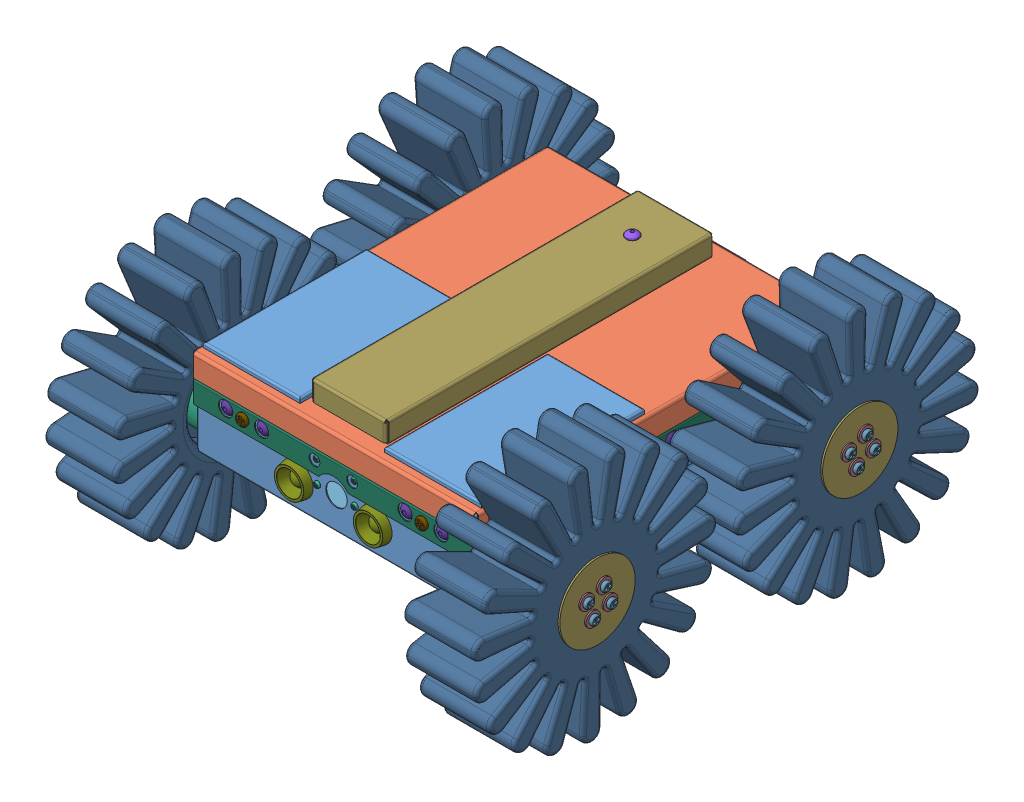
SolidWorks assembly GB0814, configuration Default. Lengths in mm. (continued)
Mates (geometry in assembly coordinates): (continued)
- Concentric111: concentric anti-aligned: cylinder of servo.fixture-1 through (144.387 0 47.956) axis (0 1 0) radius 2; cylinder of 4mm.rivet-1 through (144.387 -2.1069 47.956) axis (0 -1 0) radius 1.9261
- Concentric112: concentric anti-aligned: cylinder of servo.fixture-1 through (144.387 0 27.956) axis (0 1 0) radius 2; cylinder of 4mm.rivet-3 through (144.387 -2.1069 27.956) axis (0 -1 0) radius 1.9261
- Concentric113: concentric anti-aligned: cylinder of servo.fixture-1 through (144.387 0 7.956) axis (0 1 0) radius 2; cylinder of 4mm.rivet-2 through (144.387 -2.1069 7.956) axis (0 -1 0) radius 1.9261
- Coincident131: coincident anti-aligned: plane of case.bottom-1 through (0 -0.5 0) normal (0 -1 0); plane of 4mm.rivet-2 through (144.3664 -0.5 7.9425) normal (0 1 0)
- Coincident132: coincident anti-aligned: plane of case.bottom-1 through (0 -0.5 0) normal (0 -1 0); plane of 4mm.rivet-3 through (144.3664 -0.5 27.9425) normal (0 1 0)
- Coincident133: coincident anti-aligned: plane of case.bottom-1 through (0 -0.5 0) normal (0 -1 0); plane of 4mm.rivet-1 through (144.3664 -0.5 47.9425) normal (0 1 0)
- Coincident134: coincident anti-aligned: plane of case.bottom-1 through (0 0 0) normal (0 1 0); plane of servo.fixture-2 through (135.0187 0 151.7511) normal (0 -1 0)
- Coincident135: coincident anti-aligned: plane of SM4315R-4 through (137.0187 21 161.9111) normal (-1 0 0); plane of servo.fixture-2 through (137.0187 19 151.7511) normal (1 0 0)
- Concentric114: concentric aligned: cylinder of SM4315R-4 through (139.4 26.08 175.8811) axis (-1 0 0) radius 2.2606; cylinder of servo.fixture-2 through (153.0188 26.08 175.8811) axis (-1 0 0) radius 1.5
- Concentric115: concentric anti-aligned: cylinder of SM4315R-4 through (139.4 26.08 175.8811) axis (-1 0 0) radius 2.2606; cylinder of m3.screw.10mm-12 through (129.4 26.08 175.8811) axis (1 0 0) radius 1.5
- Coincident136: coincident anti-aligned: plane of SM4315R-4 through (139.4 21 161.9111) normal (1 0 0); plane of m3.screw.10mm-12 through (139.4 26.0936 175.8675) normal (-1 0 0)
- Concentric116: concentric anti-aligned: cylinder of SM4315R-4 through (139.4 15.92 175.8811) axis (-1 0 0) radius 2.2606; cylinder of m3.screw.10mm-9 through (129.4 15.92 175.8811) axis (1 0 0) radius 1.5
- Coincident137: coincident anti-aligned: plane of SM4315R-4 through (139.4 21 161.9111) normal (1 0 0); plane of m3.screw.10mm-9 through (139.4 15.9336 175.8675) normal (-1 0 0)
- Concentric117: concentric anti-aligned: cylinder of SM4315R-4 through (139.4 15.92 127.6211) axis (-1 0 0) radius 2.2606; cylinder of m3.screw.10mm-10 through (129.4 15.92 127.6211) axis (1 0 0) radius 1.5
- Concentric118: concentric anti-aligned: cylinder of SM4315R-4 through (139.4 26.08 127.6211) axis (-1 0 0) radius 2.2606; cylinder of m3.screw.10mm-11 through (129.4 26.08 127.6211) axis (1 0 0) radius 1.5
- Coincident138: coincident anti-aligned: plane of SM4315R-4 through (139.4 21 161.9111) normal (1 0 0); plane of m3.screw.10mm-11 through (139.4 26.0936 127.6075) normal (-1 0 0)
- Coincident139: coincident anti-aligned: plane of SM4315R-4 through (139.4 21 161.9111) normal (1 0 0); plane of m3.screw.10mm-10 through (139.4 15.9336 127.6075) normal (-1 0 0)
- Concentric119: concentric anti-aligned: cylinder of m3.screw.10mm-11 through (129.4 26.08 127.6211) axis (1 0 0) radius 1.5; cylinder of self.stop.nut.m3-25 through (135.0187 26.08 127.6211) axis (-1 0 0) radius 1.5
- Coincident140: coincident anti-aligned: plane of servo.fixture-2 through (135.0187 19 151.7511) normal (-1 0 0); plane of self.stop.nut.m3-25 through (135.0187 26.08 127.6211) normal (1 0 0)
- Concentric120: concentric anti-aligned: cylinder of m3.screw.10mm-10 through (129.4 15.92 127.6211) axis (1 0 0) radius 1.5; cylinder of self.stop.nut.m3-23 through (135.0187 15.92 127.6211) axis (-1 0 0) radius 1.5
- Coincident141: coincident anti-aligned: plane of servo.fixture-2 through (135.0187 19 151.7511) normal (-1 0 0); plane of self.stop.nut.m3-23 through (135.0187 15.92 127.6211) normal (1 0 0)
- Concentric121: concentric anti-aligned: cylinder of m3.screw.10mm-9 through (129.4 15.92 175.8811) axis (1 0 0) radius 1.5; cylinder of self.stop.nut.m3-24 through (135.0187 15.92 175.8811) axis (-1 0 0) radius 1.5
- Coincident142: coincident anti-aligned: plane of servo.fixture-2 through (135.0187 19 151.7511) normal (-1 0 0); plane of self.stop.nut.m3-24 through (135.0187 15.92 175.8811) normal (1 0 0)
- Concentric122: concentric anti-aligned: cylinder of m3.screw.10mm-12 through (129.4 26.08 175.8811) axis (1 0 0) radius 1.5; cylinder of self.stop.nut.m3-22 through (135.0187 26.08 175.8811) axis (-1 0 0) radius 1.5
- Coincident143: coincident anti-aligned: plane of servo.fixture-2 through (135.0187 19 151.7511) normal (-1 0 0); plane of self.stop.nut.m3-22 through (135.0187 26.08 175.8811) normal (1 0 0)
- Concentric123: concentric anti-aligned: cylinder of servo.fixture-2 through (144.387 0 171.7511) axis (0 1 0) radius 2; cylinder of 4mm.rivet-6 through (144.387 -2.1069 171.7511) axis (0 -1 0) radius 1.9261
- Concentric124: concentric anti-aligned: cylinder of servo.fixture-2 through (144.387 0 151.7511) axis (0 1 0) radius 2; cylinder of 4mm.rivet-5 through (144.387 -2.1069 151.7511) axis (0 -1 0) radius 1.9261
- Concentric125: concentric anti-aligned: cylinder of servo.fixture-2 through (144.387 0 131.7511) axis (0 1 0) radius 2; cylinder of 4mm.rivet-4 through (144.387 -2.1069 131.7511) axis (0 -1 0) radius 1.9261
- Coincident144: coincident anti-aligned: plane of case.bottom-1 through (0 -0.5 0) normal (0 -1 0); plane of 4mm.rivet-6 through (144.3664 -0.5 171.7376) normal (0 1 0)
- Coincident145: coincident anti-aligned: plane of case.bottom-1 through (0 -0.5 0) normal (0 -1 0); plane of 4mm.rivet-4 through (144.3664 -0.5 131.7376) normal (0 1 0)
- Coincident146: coincident anti-aligned: plane of case.bottom-1 through (0 -0.5 0) normal (0 -1 0); plane of 4mm.rivet-5 through (144.3664 -0.5 151.7376) normal (0 1 0)
- Coincident147: coincident anti-aligned: plane of case.bottom-1 through (0 0 0) normal (0 1 0); plane of servo.fixture-3 through (19.9812 0 151.7511) normal (0 -1 0)
- Coincident148: coincident anti-aligned: plane of SM4315R-1 through (17.9812 21 161.9111) normal (1 0 0); plane of servo.fixture-3 through (17.9812 19 151.7511) normal (-1 0 0)
- Concentric126: concentric aligned: cylinder of SM4315R-1 through (15.6 26.08 127.6211) axis (1 0 0) radius 2.2606; cylinder of servo.fixture-3 through (1.9812 26.08 127.6211) axis (1 0 0) radius 1.5
- Coincident149: coincident anti-aligned: plane of case.bottom-1 through (0 0 0) normal (0 1 0); plane of servo.fixture-4 through (19.9812 0 27.956) normal (0 -1 0)
- Coincident150: coincident anti-aligned: plane of SM4315R-2 through (17.9812 21 17.796) normal (1 0 0); plane of servo.fixture-4 through (17.9812 19 27.956) normal (-1 0 0)
- Concentric127: concentric aligned: cylinder of SM4315R-2 through (15.6 26.08 3.826) axis (1 0 0) radius 2.2606; cylinder of servo.fixture-4 through (1.9812 26.08 3.826) axis (1 0 0) radius 1.5
- Coincident151: coincident anti-aligned: plane of case.bottom-1 through (0 -0.5 0) normal (0 -1 0); plane of 4mm.rivet-9 through (10.5923 -0.5 47.9425) normal (0 1 0)
- Coincident152: coincident anti-aligned: plane of case.bottom-1 through (0 -0.5 0) normal (0 -1 0); plane of 4mm.rivet-8 through (10.5923 -0.5 27.9425) normal (0 1 0)
- Coincident153: coincident anti-aligned: plane of case.bottom-1 through (0 -0.5 0) normal (0 -1 0); plane of 4mm.rivet-7 through (10.5923 -0.5 7.9425) normal (0 1 0)
- Concentric128: concentric anti-aligned: cylinder of servo.fixture-4 through (10.6129 0 47.956) axis (0 1 0) radius 2; cylinder of 4mm.rivet-9 through (10.6129 -2.1069 47.956) axis (0 -1 0) radius 1.9261
- Concentric129: concentric anti-aligned: cylinder of servo.fixture-4 through (10.6129 0 27.956) axis (0 1 0) radius 2; cylinder of 4mm.rivet-8 through (10.6129 -2.1069 27.956) axis (0 -1 0) radius 1.9261
- Concentric130: concentric anti-aligned: cylinder of servo.fixture-4 through (10.6129 0 7.956) axis (0 1 0) radius 2; cylinder of 4mm.rivet-7 through (10.6129 -2.1069 7.956) axis (0 -1 0) radius 1.9261
- Coincident154: coincident anti-aligned: plane of case.bottom-1 through (0 -0.5 0) normal (0 -1 0); plane of 4mm.rivet-12 through (10.5923 -0.5 171.7376) normal (0 1 0)
- Coincident155: coincident anti-aligned: plane of case.bottom-1 through (0 -0.5 0) normal (0 -1 0); plane of 4mm.rivet-11 through (10.5923 -0.5 151.7376) normal (0 1 0)
- Coincident156: coincident anti-aligned: plane of case.bottom-1 through (0 -0.5 0) normal (0 -1 0); plane of 4mm.rivet-10 through (10.5923 -0.5 131.7376) normal (0 1 0)
- Concentric131: concentric anti-aligned: cylinder of servo.fixture-3 through (10.6129 0 171.7511) axis (0 1 0) radius 2; cylinder of 4mm.rivet-12 through (10.6129 -2.1069 171.7511) axis (0 -1 0) radius 1.9261
- Concentric132: concentric anti-aligned: cylinder of servo.fixture-3 through (10.6129 0 151.7511) axis (0 1 0) radius 2; cylinder of 4mm.rivet-11 through (10.6129 -2.1069 151.7511) axis (0 -1 0) radius 1.9261
- Concentric133: concentric anti-aligned: cylinder of servo.fixture-3 through (10.6129 0 131.7511) axis (0 1 0) radius 2; cylinder of 4mm.rivet-10 through (10.6129 -2.1069 131.7511) axis (0 -1 0) radius 1.9261
- Concentric134: concentric anti-aligned: cylinder of servo.fixture-4 through (1.9812 15.92 3.826) axis (1 0 0) radius 1.5; cylinder of m3.screw.10mm-13 through (25.6 15.92 3.826) axis (-1 0 0) radius 1.5
- Concentric135: concentric anti-aligned: cylinder of servo.fixture-4 through (1.9812 26.08 3.826) axis (1 0 0) radius 1.5; cylinder of m3.screw.10mm-14 through (25.6 26.08 3.826) axis (-1 0 0) radius 1.5
- Concentric136: concentric anti-aligned: cylinder of servo.fixture-4 through (1.9812 15.92 52.086) axis (1 0 0) radius 1.5; cylinder of m3.screw.10mm-15 through (25.6 15.92 52.086) axis (-1 0 0) radius 1.5
- Concentric137: concentric anti-aligned: cylinder of servo.fixture-4 through (1.9812 26.08 52.086) axis (1 0 0) radius 1.5; cylinder of m3.screw.10mm-16 through (25.6 26.08 52.086) axis (-1 0 0) radius 1.5
- Coincident157: coincident anti-aligned: plane of SM4315R-2 through (15.6 21 17.796) normal (-1 0 0); plane of m3.screw.10mm-14 through (15.6 26.0936 3.8396) normal (1 0 0)
- Coincident158: coincident anti-aligned: plane of SM4315R-2 through (15.6 21 17.796) normal (-1 0 0); plane of m3.screw.10mm-13 through (15.6 15.9336 3.8396) normal (1 0 0)
- Coincident159: coincident anti-aligned: plane of SM4315R-2 through (15.6 21 17.796) normal (-1 0 0); plane of m3.screw.10mm-16 through (15.6 26.0936 52.0996) normal (1 0 0)
- Coincident160: coincident anti-aligned: plane of SM4315R-2 through (15.6 21 17.796) normal (-1 0 0); plane of m3.screw.10mm-15 through (15.6 15.9336 52.0996) normal (1 0 0)
- Concentric138: concentric anti-aligned: cylinder of m3.screw.10mm-13 through (25.6 15.92 3.826) axis (-1 0 0) radius 1.5; cylinder of self.stop.nut.m3-26 through (19.9812 15.92 3.826) axis (1 0 0) radius 1.5
- Concentric139: concentric anti-aligned: cylinder of m3.screw.10mm-14 through (25.6 26.08 3.826) axis (-1 0 0) radius 1.5; cylinder of self.stop.nut.m3-27 through (19.9812 26.08 3.826) axis (1 0 0) radius 1.5
- Concentric140: concentric anti-aligned: cylinder of m3.screw.10mm-15 through (25.6 15.92 52.086) axis (-1 0 0) radius 1.5; cylinder of self.stop.nut.m3-28 through (19.9812 15.92 52.086) axis (1 0 0) radius 1.5
- Concentric141: concentric anti-aligned: cylinder of m3.screw.10mm-16 through (25.6 26.08 52.086) axis (-1 0 0) radius 1.5; cylinder of self.stop.nut.m3-29 through (19.9812 26.08 52.086) axis (1 0 0) radius 1.5
- Coincident161: coincident anti-aligned: plane of servo.fixture-4 through (19.9812 19 27.956) normal (1 0 0); plane of self.stop.nut.m3-29 through (19.9812 26.08 52.086) normal (-1 0 0)
- Coincident162: coincident anti-aligned: plane of servo.fixture-4 through (19.9812 19 27.956) normal (1 0 0); plane of self.stop.nut.m3-28 through (19.9812 15.92 52.086) normal (-1 0 0)
- Coincident163: coincident anti-aligned: plane of servo.fixture-4 through (19.9812 19 27.956) normal (1 0 0); plane of self.stop.nut.m3-27 through (19.9812 26.08 3.826) normal (-1 0 0)
- Coincident164: coincident anti-aligned: plane of servo.fixture-4 through (19.9812 19 27.956) normal (1 0 0); plane of self.stop.nut.m3-26 through (19.9812 15.92 3.826) normal (-1 0 0)
- Concentric142: concentric anti-aligned: cylinder of servo.fixture-3 through (1.9812 15.92 127.6211) axis (1 0 0) radius 1.5; cylinder of m3.screw.10mm-17 through (25.6 15.92 127.6211) axis (-1 0 0) radius 1.5
- Concentric143: concentric anti-aligned: cylinder of servo.fixture-3 through (1.9812 26.08 127.6211) axis (1 0 0) radius 1.5; cylinder of m3.screw.10mm-18 through (25.6 26.08 127.6211) axis (-1 0 0) radius 1.5
- Concentric144: concentric anti-aligned: cylinder of servo.fixture-3 through (1.9812 15.92 175.8811) axis (1 0 0) radius 1.5; cylinder of m3.screw.10mm-20 through (25.6 15.92 175.8811) axis (-1 0 0) radius 1.5
- Concentric145: concentric anti-aligned: cylinder of servo.fixture-3 through (1.9812 26.08 175.8811) axis (1 0 0) radius 1.5; cylinder of m3.screw.10mm-19 through (25.6 26.08 175.8811) axis (-1 0 0) radius 1.5
- Coincident165: coincident anti-aligned: plane of SM4315R-1 through (15.6 21 161.9111) normal (-1 0 0); plane of m3.screw.10mm-18 through (15.6 26.0936 127.6347) normal (1 0 0)
- Coincident166: coincident anti-aligned: plane of SM4315R-1 through (15.6 21 161.9111) normal (-1 0 0); plane of m3.screw.10mm-17 through (15.6 15.9336 127.6347) normal (1 0 0)
- Coincident167: coincident anti-aligned: plane of SM4315R-1 through (15.6 21 161.9111) normal (-1 0 0); plane of m3.screw.10mm-19 through (15.6 26.0936 175.8947) normal (1 0 0)
- Coincident168: coincident anti-aligned: plane of SM4315R-1 through (15.6 21 161.9111) normal (-1 0 0); plane of m3.screw.10mm-20 through (15.6 15.9336 175.8947) normal (1 0 0)
- Concentric146: concentric anti-aligned: cylinder of m3.screw.10mm-18 through (25.6 26.08 127.6211) axis (-1 0 0) radius 1.5; cylinder of self.stop.nut.m3-30 through (19.9812 26.08 127.6211) axis (1 0 0) radius 1.5
- Concentric147: concentric anti-aligned: cylinder of m3.screw.10mm-17 through (25.6 15.92 127.6211) axis (-1 0 0) radius 1.5; cylinder of self.stop.nut.m3-31 through (19.9812 15.92 127.6211) axis (1 0 0) radius 1.5
- Concentric148: concentric anti-aligned: cylinder of m3.screw.10mm-20 through (25.6 15.92 175.8811) axis (-1 0 0) radius 1.5; cylinder of self.stop.nut.m3-33 through (19.9812 15.92 175.8811) axis (1 0 0) radius 1.5
- Concentric149: concentric anti-aligned: cylinder of m3.screw.10mm-19 through (25.6 26.08 175.8811) axis (-1 0 0) radius 1.5; cylinder of self.stop.nut.m3-32 through (19.9812 26.08 175.8811) axis (1 0 0) radius 1.5
- Coincident169: coincident anti-aligned: plane of servo.fixture-3 through (19.9812 19 151.7511) normal (1 0 0); plane of self.stop.nut.m3-32 through (19.9812 26.08 175.8811) normal (-1 0 0)
- Coincident170: coincident anti-aligned: plane of servo.fixture-3 through (19.9812 19 151.7511) normal (1 0 0); plane of self.stop.nut.m3-33 through (19.9812 15.92 175.8811) normal (-1 0 0)
- Coincident171: coincident anti-aligned: plane of servo.fixture-3 through (19.9812 19 151.7511) normal (1 0 0); plane of self.stop.nut.m3-30 through (19.9812 26.08 127.6211) normal (-1 0 0)
- Coincident172: coincident anti-aligned: plane of servo.fixture-3 through (19.9812 19 151.7511) normal (1 0 0); plane of self.stop.nut.m3-31 through (19.9812 15.92 127.6211) normal (-1 0 0)
- Parallel13: parallel anti-aligned: plane of RasPi_Camera-1/RasPi_Camera_Board-1 through (77.5 24.1874 177.7694) normal (0 0 1); plane of camera.glass-1 through (77.5 26.6874 183.0711) normal (0 0 -1)
- Distance25: distance = 7.5 mm aligned: plane of camera.glass-1 through (97.5 8.2612 187.0711) normal (1 0 0); plane of RasPi_Camera-1/RasPi_Camera_Board-1 through (90 38.6874 176.8694) normal (1 0 0)
- Distance27: distance = 3 mm aligned: plane of camera.glass-1 through (97.5 41.6874 187.0711) normal (0 1 0); plane of RasPi_Camera-1/RasPi_Camera_Board-1 through (65 38.6874 176.8694) normal (0 1 0)
- Coincident173: coincident anti-aligned: plane of RasPi_Camera-1/OVA5647-1/OVA5647_Lens-1 through (76.5 24.1874 183.0711) normal (0 0 1); plane of camera.glass-1 through (77.5 26.6874 183.0711) normal (0 0 -1)
- Concentric150: concentric anti-aligned: cylinder of case.bottom-1 through (77.5 24.1874 177.5711) axis (0 0 1) radius 6; cylinder of ? through (77.5 24.1874 182.2711) axis (0 0 -1) radius 3.8
- Coincident174: coincident anti-aligned: plane of case.bottom-1 through (0 0 187.0711) normal (0 0 -1); plane of camera.glass-1 through (77.5 26.6874 187.0711) normal (0 0 1)
- Parallel14: parallel aligned: plane of case.bottom-1 through (154.5 42 187.5711) normal (0 1 0); plane of camera.glass-1 through (97.5 41.6874 187.0711) normal (0 1 0)
- Concentric151: concentric anti-aligned: cylinder of case.bottom-1 through (88 36.6874 192.0711) axis (0 0 -1) radius 1.05; cylinder of m2.screw.15mm-4 through (88 36.6874 172.5711) axis (0 0 1) radius 1
- Coincident175: coincident anti-aligned: plane of case.bottom-1 through (0 0 187.5711) normal (0 0 1); plane of m2.screw.15mm-4 through (88.0073 36.7052 187.5711) normal (0 0 -1)
- Concentric152: concentric anti-aligned: cylinder of case.bottom-1 through (67 36.6874 192.0711) axis (0 0 -1) radius 1.05; cylinder of m2.screw.15mm-1 through (67 36.6874 172.5711) axis (0 0 1) radius 1
- Concentric153: concentric anti-aligned: cylinder of case.bottom-1 through (88 24.1874 192.0711) axis (0 0 -1) radius 1.05; cylinder of m2.screw.15mm-3 through (88 24.1874 172.5711) axis (0 0 1) radius 1
- Concentric154: concentric anti-aligned: cylinder of case.bottom-1 through (67 24.1874 192.0711) axis (0 0 -1) radius 1.05; cylinder of m2.screw.15mm-2 through (67 24.1874 172.5711) axis (0 0 1) radius 1
- Coincident176: coincident anti-aligned: plane of case.bottom-1 through (0 0 187.5711) normal (0 0 1); plane of m2.screw.15mm-3 through (88.0073 24.2052 187.5711) normal (0 0 -1)
- Coincident177: coincident anti-aligned: plane of case.bottom-1 through (0 0 187.5711) normal (0 0 1); plane of m2.screw.15mm-2 through (67.0073 24.2052 187.5711) normal (0 0 -1)
- Coincident178: coincident anti-aligned: plane of case.bottom-1 through (0 0 187.5711) normal (0 0 1); plane of m2.screw.15mm-1 through (67.0073 36.7052 187.5711) normal (0 0 -1)
- Concentric155: concentric anti-aligned: cylinder of m2.screw.15mm-4 through (88 36.6874 172.5711) axis (0 0 1) radius 1; cylinder of nut.m2-1 through (88 36.6874 176.8694) axis (0 0 -1) radius 1
- Concentric156: concentric anti-aligned: cylinder of m2.screw.15mm-3 through (88 24.1874 172.5711) axis (0 0 1) radius 1; cylinder of nut.m2-2 through (88 24.1874 176.8694) axis (0 0 -1) radius 1
- Concentric157: concentric anti-aligned: cylinder of m2.screw.15mm-2 through (67 24.1874 172.5711) axis (0 0 1) radius 1; cylinder of nut.m2-3 through (67 24.1874 176.8694) axis (0 0 -1) radius 1
- Concentric158: concentric anti-aligned: cylinder of m2.screw.15mm-1 through (67 36.6874 172.5711) axis (0 0 1) radius 1; cylinder of nut.m2-4 through (67 36.6874 176.8694) axis (0 0 -1) radius 1
- Coincident179: coincident anti-aligned: plane of RasPi_Camera-1/RasPi_Camera_Board-1 through (77.5 24.1874 176.8694) normal (0 0 -1); plane of nut.m2-1 through (88 36.6874 176.8694) normal (0 0 1)
- Coincident180: coincident anti-aligned: plane of RasPi_Camera-1/RasPi_Camera_Board-1 through (77.5 24.1874 176.8694) normal (0 0 -1); plane of nut.m2-2 through (88 24.1874 176.8694) normal (0 0 1)
- Coincident181: coincident anti-aligned: plane of RasPi_Camera-1/RasPi_Camera_Board-1 through (77.5 24.1874 176.8694) normal (0 0 -1); plane of nut.m2-4 through (67 36.6874 176.8694) normal (0 0 1)
- Coincident182: coincident anti-aligned: plane of RasPi_Camera-1/RasPi_Camera_Board-1 through (77.5 24.1874 176.8694) normal (0 0 -1); plane of nut.m2-3 through (67 24.1874 176.8694) normal (0 0 1)
- Concentric159: concentric anti-aligned: cylinder of m2.screw.15mm-4 through (88 36.6874 172.5711) axis (0 0 1) radius 1; cylinder of m2.pillar-4 through (88 36.6874 183.0711) axis (0 0 -1) radius 1
- Concentric160: concentric anti-aligned: cylinder of m2.screw.15mm-3 through (88 24.1874 172.5711) axis (0 0 1) radius 1; cylinder of m2.pillar-3 through (88 24.1874 183.0711) axis (0 0 -1) radius 1
- Concentric161: concentric anti-aligned: cylinder of m2.screw.15mm-2 through (67 24.1874 172.5711) axis (0 0 1) radius 1; cylinder of m2.pillar-2 through (67 24.1874 183.0711) axis (0 0 -1) radius 1
- Concentric162: concentric anti-aligned: cylinder of m2.screw.15mm-1 through (67 36.6874 172.5711) axis (0 0 1) radius 1; cylinder of m2.pillar-1 through (67 36.6874 183.0711) axis (0 0 -1) radius 1
- Coincident183: coincident anti-aligned: plane of camera.glass-1 through (77.5 26.6874 183.0711) normal (0 0 -1); plane of m2.pillar-4 through (88 36.6874 183.0711) normal (0 0 1)
- Coincident184: coincident anti-aligned: plane of camera.glass-1 through (77.5 26.6874 183.0711) normal (0 0 -1); plane of m2.pillar-3 through (88 24.1874 183.0711) normal (0 0 1)
- Coincident185: coincident anti-aligned: plane of camera.glass-1 through (77.5 26.6874 183.0711) normal (0 0 -1); plane of m2.pillar-2 through (67 24.1874 183.0711) normal (0 0 1)
- Coincident186: coincident anti-aligned: plane of camera.glass-1 through (77.5 26.6874 183.0711) normal (0 0 -1); plane of m2.pillar-1 through (67 36.6874 183.0711) normal (0 0 1)
- Lock13: lock: unknown of RasPi_Camera-1/RasPi_Camera_Board-1; unknown of camera.cable-1
- Tangent22: tangent anti-aligned: plane of wheel.hub-2 through (-8.5 21 163.0711) normal (-1 0 0); unknown of ball.4mm-64
- Tangent23: tangent anti-aligned: unknown of ball.4mm-64; plane of flange-2 through (-12.5 21 163.0711) normal (1 0 0)
- Concentric163: concentric aligned: cylinder of flange-3 through (170.5 21 163.0711) axis (-1 0 0) radius 20; cylinder of wheel.assembly-1/wheel-1 through (170.5 21 163.0711) axis (-1 0 0) radius 25
- Concentric164: concentric aligned: cylinder of wheel.hub-3 through (161.5 17.7804 156.5752) axis (1 0 0) radius 1.5; cylinder of wheel.assembly-1/m3.screw.36mm-1 through (163.3 17.7804 156.5752) axis (1 0 0) radius 1.5
- Coincident187: coincident anti-aligned: plane of wheel.hub-3 through (171.5 21 163.0711) normal (1 0 0); plane of wheel.assembly-1/wheel.spacer-1 through (171.5 21 163.0711) normal (-1 0 0)
- Concentric165: concentric aligned: cylinder of wheel.hub-1 through (-6.5 28.2497 16.7014) axis (-1 0 0) radius 1.5; cylinder of wheel.assembly-2/m3.screw.36mm-3 through (-8.3 28.2497 16.7014) axis (-1 0 0) radius 1.5
- Concentric166: concentric aligned: cylinder of flange-1 through (-15.5 21.0015 16.8638) axis (1 0 0) radius 20; cylinder of wheel.assembly-2/wheel-1 through (-15.5 21.0015 16.8638) axis (1 0 0) radius 25
- Coincident188: coincident anti-aligned: plane of wheel.hub-1 through (-16.5 21 16.636) normal (-1 0 0); plane of wheel.assembly-2/wheel.spacer-1 through (-16.5 21.0015 16.8638) normal (1 0 0)
- Concentric167: concentric aligned: cylinder of wheel.hub-2 through (-6.5 27.9309 165.1983) axis (-1 0 0) radius 1.5; cylinder of wheel.assembly-3/m3.screw.36mm-3 through (-8.3 27.9309 165.1983) axis (-1 0 0) radius 1.5
- Concentric168: concentric aligned: cylinder of flange-2 through (-15.5 21 163.0711) axis (1 0 0) radius 20; cylinder of wheel.assembly-3/wheel-1 through (-15.5 21 163.0711) axis (1 0 0) radius 25
- Coincident189: coincident anti-aligned: plane of wheel.hub-2 through (-16.5 21 163.0711) normal (-1 0 0); plane of wheel.assembly-3/wheel.spacer-1 through (-16.5 21 163.0711) normal (1 0 0)
- Concentric169: concentric aligned: cylinder of wheel.hub-4 through (161.5 27.8192 14.174) axis (1 0 0) radius 1.5; cylinder of wheel.assembly-4/m3.screw.36mm-4 through (163.3 27.8192 14.174) axis (1 0 0) radius 1.5
- Concentric170: concentric aligned: cylinder of flange-4 through (170.5 21 16.636) axis (-1 0 0) radius 20; cylinder of wheel.assembly-4/wheel-1 through (170.5 21 16.636) axis (-1 0 0) radius 25
- Coincident190: coincident anti-aligned: plane of wheel.hub-4 through (171.5 21 16.636) normal (1 0 0); plane of wheel.assembly-4/wheel.spacer-1 through (171.5 21 16.636) normal (-1 0 0)
- Coincident191: coincident anti-aligned: plane of case.bottom-1 through (154.5 42 187.5711) normal (0 1 0); plane of case.cap-1 through (155.5 42 -8.1489) normal (0 -1 0)
- Parallel15: parallel aligned: plane of case.bottom-1 through (155.5 0 0) normal (1 0 0); plane of case.cap-1 through (157 42 -8.1489) normal (1 0 0)
- Distance28: distance = 1 mm anti-aligned: plane of case.bottom-1 through (-0.5 0 0) normal (-1 0 0); plane of case.cap-1 through (-1.5 42 -8.1489) normal (1 0 0)
- Distance29: distance = 1.28 mm anti-aligned: plane of case.cap-1 through (155.5 42 188.8511) normal (0 0 -1); plane of case.bottom-1 through (0 0 187.5711) normal (0 0 1)
- Lock14: lock: unknown of case.bottom-1; unknown of cap.fixture-1
- Lock15: lock: unknown of case.bottom-1; unknown of cap.fixture-2
- Lock16: lock: unknown of case.bottom-1; unknown of cap.fixture-3
- Lock17: lock: unknown of case.bottom-1; unknown of cap.fixture-4
- Lock18: lock: unknown of case.bottom-1; unknown of cap.fixture-5
- Lock19: lock: unknown of case.bottom-1; unknown of cap.fixture-6
- Concentric177: concentric anti-aligned: cylinder of cap.fixture-6 through (137.5 36.75 -7.364) axis (0 0 1) radius 2; cylinder of 4mmx8mm.rivet-1 through (137.5 36.75 -6.5518) axis (0 0 -1) radius 1.9261
- Coincident198: coincident anti-aligned: plane of case.bottom-1 through (0 0.2929 -7.864) normal (0 0 -1); plane of 4mmx8mm.rivet-1 through (137.5247 36.75 -7.864) normal (0 0 1)
- Concentric178: concentric anti-aligned: cylinder of cap.fixture-6 through (117.5 36.75 -7.364) axis (0 0 1) radius 2; cylinder of 4mmx8mm.rivet-2 through (117.5 36.75 -6.5518) axis (0 0 -1) radius 1.9261
- Coincident199: coincident anti-aligned: plane of case.bottom-1 through (0 0.2929 -7.864) normal (0 0 -1); plane of 4mmx8mm.rivet-2 through (117.5247 36.75 -7.864) normal (0 0 1)
- Concentric179: concentric anti-aligned: cylinder of cap.fixture-5 through (37.5 36.75 -7.364) axis (0 0 1) radius 2; cylinder of 4mmx8mm.rivet-3 through (37.5 36.75 -6.5518) axis (0 0 -1) radius 1.9261
- Concentric180: concentric anti-aligned: cylinder of cap.fixture-5 through (17.5 36.75 -7.364) axis (0 0 1) radius 2; cylinder of 4mmx8mm.rivet-4 through (17.5 36.75 -6.5518) axis (0 0 -1) radius 1.9261
- Coincident200: coincident anti-aligned: plane of case.bottom-1 through (0 0.2929 -7.864) normal (0 0 -1); plane of 4mmx8mm.rivet-3 through (37.5247 36.75 -7.864) normal (0 0 1)
- Coincident201: coincident anti-aligned: plane of case.bottom-1 through (0 0.2929 -7.864) normal (0 0 -1); plane of 4mmx8mm.rivet-4 through (17.5247 36.75 -7.864) normal (0 0 1)
- Concentric181: concentric anti-aligned: cylinder of cap.fixture-4 through (17.5 36.75 187.0711) axis (0 0 -1) radius 2; cylinder of 4mmx8mm.rivet-5 through (17.5 36.75 186.2589) axis (0 0 1) radius 1.9261
- Concentric182: concentric anti-aligned: cylinder of cap.fixture-4 through (37.5 36.75 187.0711) axis (0 0 -1) radius 2; cylinder of 4mmx8mm.rivet-6 through (37.5 36.75 186.2589) axis (0 0 1) radius 1.9261
- Concentric183: concentric anti-aligned: cylinder of cap.fixture-3 through (117.5 36.75 187.0711) axis (0 0 -1) radius 2; cylinder of 4mmx8mm.rivet-7 through (117.5 36.75 186.2589) axis (0 0 1) radius 1.9261
- Concentric184: concentric anti-aligned: cylinder of cap.fixture-3 through (137.5 36.75 187.0711) axis (0 0 -1) radius 2; cylinder of 4mmx8mm.rivet-8 through (137.5 36.75 186.2589) axis (0 0 1) radius 1.9261
- Coincident202: coincident anti-aligned: plane of case.bottom-1 through (0 0 187.5711) normal (0 0 1); plane of 4mmx8mm.rivet-7 through (117.5091 36.7271 187.5711) normal (0 0 -1)
- Coincident203: coincident anti-aligned: plane of case.bottom-1 through (0 0 187.5711) normal (0 0 1); plane of 4mmx8mm.rivet-8 through (137.518 36.7332 187.5711) normal (0 0 -1)
- Coincident204: coincident anti-aligned: plane of case.bottom-1 through (0 0 187.5711) normal (0 0 1); plane of 4mmx8mm.rivet-6 through (37.5241 36.7552 187.5711) normal (0 0 -1)
- Coincident205: coincident anti-aligned: plane of case.bottom-1 through (0 0 187.5711) normal (0 0 1); plane of 4mmx8mm.rivet-5 through (17.5023 36.7254 187.5711) normal (0 0 -1)
- Concentric185: concentric anti-aligned: cylinder of cap.fixture-2 through (0 36.8819 79.9679) axis (1 0 0) radius 2; cylinder of 4mmx8mm.rivet-9 through (0.8122 36.8819 79.9679) axis (-1 0 0) radius 1.9261
- Concentric186: concentric anti-aligned: cylinder of cap.fixture-2 through (0 36.8819 99.9679) axis (1 0 0) radius 2; cylinder of 4mmx8mm.rivet-10 through (0.8122 36.8819 99.9679) axis (-1 0 0) radius 1.9261
- Coincident206: coincident anti-aligned: plane of case.bottom-1 through (-0.5 0 0) normal (-1 0 0); plane of 4mmx8mm.rivet-9 through (-0.5 36.9065 79.9679) normal (1 0 0)
- Coincident207: coincident anti-aligned: plane of case.bottom-1 through (-0.5 0 0) normal (-1 0 0); plane of 4mmx8mm.rivet-10 through (-0.5 36.9065 99.9679) normal (1 0 0)
- Concentric187: concentric anti-aligned: cylinder of cap.fixture-1 through (155 36.8819 99.9679) axis (-1 0 0) radius 2; cylinder of 4mmx8mm.rivet-12 through (154.1878 36.8819 99.9679) axis (1 0 0) radius 1.9261
- Concentric188: concentric anti-aligned: cylinder of cap.fixture-1 through (155 36.8819 79.9679) axis (-1 0 0) radius 2; cylinder of 4mmx8mm.rivet-11 through (154.1878 36.8819 79.9679) axis (1 0 0) radius 1.9261
- Coincident208: coincident anti-aligned: plane of case.bottom-1 through (155.5 0 0) normal (1 0 0); plane of 4mmx8mm.rivet-12 through (155.5 36.8572 99.9679) normal (-1 0 0)
- Coincident209: coincident anti-aligned: plane of case.bottom-1 through (155.5 0 0) normal (1 0 0); plane of 4mmx8mm.rivet-11 through (155.5 36.8572 79.9679) normal (-1 0 0)
- Coincident210: coincident anti-aligned: plane of case.cap-1 through (155.5 42 -9.6489) normal (0 0 -1); plane of m4.screw.15mm-1 through (127.4864 36.7636 -9.6489) normal (0 0 1)
- Coincident211: coincident anti-aligned: plane of case.cap-1 through (155.5 42 -9.6489) normal (0 0 -1); plane of m4.screw.15mm-2 through (27.4864 36.7636 -9.6489) normal (0 0 1)
- Concentric189: concentric anti-aligned: cylinder of cap.fixture-6 through (127.5 36.75 -7.364) axis (0 0 1) radius 2; cylinder of m4.screw.15mm-1 through (127.5 36.75 5.3511) axis (0 0 -1) radius 2
- Concentric190: concentric anti-aligned: cylinder of cap.fixture-5 through (27.5 36.75 -7.364) axis (0 0 1) radius 2; cylinder of m4.screw.15mm-2 through (27.5 36.75 5.3511) axis (0 0 -1) radius 2
- Coincident212: coincident anti-aligned: plane of case.cap-1 through (155.5 42 189.3511) normal (0 0 1); plane of m4.screw.15mm-3 through (27.5073 36.7678 189.3511) normal (0 0 -1)
- Coincident213: coincident anti-aligned: plane of case.cap-1 through (155.5 42 189.3511) normal (0 0 1); plane of m4.screw.15mm-4 through (127.5073 36.7678 189.3511) normal (0 0 -1)
- Concentric191: concentric anti-aligned: cylinder of cap.fixture-4 through (27.5 36.75 187.0711) axis (0 0 -1) radius 2; cylinder of m4.screw.15mm-3 through (27.5 36.75 174.3511) axis (0 0 1) radius 2
- Concentric192: concentric anti-aligned: cylinder of cap.fixture-3 through (127.5 36.75 187.0711) axis (0 0 -1) radius 2; cylinder of m4.screw.15mm-4 through (127.5 36.75 174.3511) axis (0 0 1) radius 2
- Coincident214: coincident anti-aligned: plane of case.cap-1 through (-2 42 -8.1489) normal (-1 0 0); plane of m4.screw.15mm-5 through (-2 36.8954 89.9815) normal (1 0 0)
- Concentric193: concentric anti-aligned: cylinder of cap.fixture-2 through (0 36.8819 89.9679) axis (1 0 0) radius 2; cylinder of m4.screw.15mm-5 through (13 36.8819 89.9679) axis (-1 0 0) radius 2
- Coincident215: coincident anti-aligned: plane of case.cap-1 through (157 42 -8.1489) normal (1 0 0); plane of m4.screw.15mm-6 through (157 36.8954 89.9543) normal (-1 0 0)
- Concentric194: concentric anti-aligned: cylinder of cap.fixture-1 through (155 36.8819 89.9679) axis (-1 0 0) radius 2; cylinder of m4.screw.15mm-6 through (142 36.8819 89.9679) axis (1 0 0) radius 2
- Distance30: distance = 10 mm aligned: plane of solar.panel-3 through (147 45 93.3511) normal (1 0 0); plane of case.cap-1 through (157 42 -8.1489) normal (1 0 0)
- Distance31: distance = 10 mm aligned: plane of solar.panel-5 through (147 45 -4.6489) normal (1 0 0); plane of case.cap-1 through (157 42 -8.1489) normal (1 0 0)
- Distance32: distance = 10 mm aligned: plane of case.cap-1 through (-2 42 -8.1489) normal (-1 0 0); plane of solar.panel-2 through (8 45 93.3511) normal (-1 0 0)
- Distance33: distance = 10 mm aligned: plane of case.cap-1 through (-2 42 -8.1489) normal (-1 0 0); plane of solar.panel-4 through (8 45 -4.6489) normal (-1 0 0)
- Distance34: distance = 5 mm aligned: plane of case.cap-1 through (155.5 42 189.3511) normal (0 0 1); plane of solar.panel-2 through (8 45 184.3511) normal (0 0 1)
- Distance35: distance = 5 mm aligned: plane of case.cap-1 through (155.5 42 189.3511) normal (0 0 1); plane of solar.panel-3 through (93 45 184.3511) normal (0 0 1)
- Distance36: distance = 5 mm aligned: plane of case.cap-1 through (155.5 42 -9.6489) normal (0 0 -1); plane of solar.panel-4 through (8 45 -4.6489) normal (0 0 -1)
- Distance37: distance = 5 mm aligned: plane of case.cap-1 through (155.5 42 -9.6489) normal (0 0 -1); plane of solar.panel-5 through (93 45 -4.6489) normal (0 0 -1)
- Lock20: lock: unknown of case.cap-1; unknown of hinge.p1-1
- Concentric197: concentric anti-aligned: circle of hinge.p1-1; circle of hinge.p2-1
- Coincident222: coincident anti-aligned: plane of hinge.p1-1 through (95 39.4474 -14.6489) normal (-1 0 0); plane of hinge.p2-1 through (95 37.6036 -14.6489) normal (1 0 0)
- Coincident223: coincident anti-aligned: plane of case.over.cap-1 through (155.5 54.4828 -9.6489) normal (0 0 -1); plane of hinge.p2-1 through (47.5588 42.4828 -9.6489) normal (0 0 1)
- Lock21: lock: unknown of case.over.cap-1; unknown of hinge.p2-1
- Coincident225: coincident aligned: plane of case.cap-1 through (157 42 -8.1489) normal (1 0 0); plane of case.over.cap-1 through (157 54.4828 -8.1489) normal (1 0 0)
- Coincident227: coincident anti-aligned: plane of case.cap-1 through (155.5 42.5 -8.1489) normal (0 1 0); plane of solar.panel-3 through (120 42.5 138.8511) normal (0 -1 0)
- Coincident228: coincident anti-aligned: plane of case.cap-1 through (155.5 42.5 -8.1489) normal (0 1 0); plane of solar.panel-5 through (120 42.5 40.8511) normal (0 -1 0)
- Coincident229: coincident anti-aligned: plane of case.cap-1 through (155.5 42.5 -8.1489) normal (0 1 0); plane of solar.panel-2 through (35 42.5 138.8511) normal (0 -1 0)
- Coincident230: coincident anti-aligned: plane of case.cap-1 through (155.5 42.5 -8.1489) normal (0 1 0); plane of solar.panel-4 through (35 42.5 40.8511) normal (0 -1 0)
- Distance44: distance = 5 mm anti-aligned: plane of case.over.cap-1 through (-1.5 54.4828 -8.1489) normal (1 0 0); plane of solar.panel-8 through (3.5 51.9828 86.8511) normal (-1 0 0)
- Distance45: distance = 5 mm anti-aligned: plane of case.over.cap-1 through (155.5 54.4828 -9.1489) normal (0 0 1); plane of solar.panel-8 through (3.5 51.9828 -4.1489) normal (0 0 -1)
- Distance46: distance = 5 mm anti-aligned: plane of case.over.cap-1 through (155.5 54.4828 188.8511) normal (0 0 -1); plane of solar.panel-9 through (3.5 51.9828 183.8511) normal (0 0 1)
- Distance47: distance = 5 mm anti-aligned: plane of case.over.cap-1 through (-1.5 54.4828 -8.1489) normal (1 0 0); plane of solar.panel-9 through (3.5 51.9828 183.8511) normal (-1 0 0)
- Distance48: distance = 5 mm anti-aligned: plane of case.over.cap-1 through (156.5 54.4828 -8.1489) normal (-1 0 0); plane of solar.panel-6 through (151.5 51.9828 86.8511) normal (1 0 0)
- Distance49: distance = 5 mm anti-aligned: plane of solar.panel-6 through (97.5 51.9828 -4.1489) normal (0 0 -1); plane of case.over.cap-1 through (155.5 54.4828 -9.1489) normal (0 0 1)
- Distance50: distance = 5 mm anti-aligned: plane of solar.panel-7 through (97.5 51.9828 183.8511) normal (0 0 1); plane of case.over.cap-1 through (155.5 54.4828 188.8511) normal (0 0 -1)
- Distance51: distance = 5 mm anti-aligned: plane of case.over.cap-1 through (156.5 54.4828 -8.1489) normal (-1 0 0); plane of solar.panel-7 through (151.5 51.9828 183.8511) normal (1 0 0)
- Coincident231: coincident anti-aligned: plane of case.over.cap-1 through (155.5 54.4828 -8.1489) normal (0 -1 0); plane of solar.panel-6 through (124.5 54.4828 41.3511) normal (0 1 0)
- Coincident232: coincident anti-aligned: plane of case.over.cap-1 through (155.5 54.4828 -8.1489) normal (0 -1 0); plane of solar.panel-7 through (124.5 54.4828 138.3511) normal (0 1 0)
- Coincident233: coincident anti-aligned: plane of case.over.cap-1 through (155.5 54.4828 -8.1489) normal (0 -1 0); plane of solar.panel-8 through (30.5 54.4828 41.3511) normal (0 1 0)
- Coincident234: coincident anti-aligned: plane of case.over.cap-1 through (155.5 54.4828 -8.1489) normal (0 -1 0); plane of solar.panel-9 through (30.5 54.4828 138.3511) normal (0 1 0)
- Lock25: lock: unknown of case.over.cap-1; unknown of actuator.cap-1
- Parallel19: parallel anti-aligned: plane of case.bottom-1 through (155.5 0 0) normal (1 0 0); plane of finger.actuator.p1-1 through (70 60.1802 133.4762) normal (-1 0 0)
- Distance52: distance = 72 mm aligned: plane of finger.actuator.p1-1 through (85 60.1802 133.4762) normal (1 0 0); plane of case.cap-1 through (157 42 -8.1489) normal (1 0 0)
- Concentric198: concentric anti-aligned: cylinder of finger.actuator.p1-1 through (77.5 52.6813 133.3502) axis (0 0.016791 -0.999859) radius 4.5; cylinder of finger.actuator.p2-1 through (77.5 54.4742 26.591) axis (0 -0.016791 0.999859) radius 4.5
- Parallel20: parallel aligned: plane of finger.actuator.p1-1 through (83.5 60.4771 26.4661) normal (1 0 0); plane of finger.actuator.p2-1 through (80.5 41.1474 16.1647) normal (1 0 0)
- Coincident237: coincident: plane of case.cap-1 through (155.5 42.5 -8.1489) normal (0 1 0); plane of actuator.fixture-1 through (77.4866 42.5 165.5173) normal (0 -1 0)
- Concentric200: concentric anti-aligned: cylinder of finger.actuator.p1-1 through (81.5 51.9844 174.8444) axis (-1 0 0) radius 2.1; cylinder of actuator.fixture-1 through (72.2634 51.9844 174.8444) axis (1 0 0) radius 2
- Distance53: distance = 0.75 mm: plane of finger.actuator.p1-1 through (73.5 53.7064 167.0173) normal (-1 0 0); plane of actuator.fixture-1 through (72.75 42.5 165.5173) normal (1 0 0)
- Concentric201: concentric aligned: cylinder of case.cap-1 through (77.5 40.5 174.8444) axis (0 1 0) radius 2; cylinder of 4mmx4mm.rivet-1 through (77.5 45.6878 174.8444) axis (0 1 0) radius 1.9261
- Coincident239: coincident anti-aligned: plane of actuator.fixture-1 through (77.5 43 174.8444) normal (0 1 0); plane of 4mmx4mm.rivet-1 through (77.5247 43 174.8444) normal (0 -1 0)
- Coincident241: coincident anti-aligned: plane of actuator.fixture-1 through (72.2634 42.5 174.8444) normal (-1 0 0); plane of self.stop.nut.m4-1 through (72.2634 51.9844 174.8444) normal (1 0 0)
- Concentric206: concentric anti-aligned: cylinder of finger.actuator.p1-1 through (81.5 51.9844 174.8444) axis (-1 0 0) radius 2.1; cylinder of m4.screw.18-1 through (64.7366 51.9844 174.8444) axis (1 0 0) radius 2
- Concentric207: concentric anti-aligned: cylinder of self.stop.nut.m4-1 through (72.2634 51.9844 174.8444) axis (-1 0 0) radius 2; cylinder of m4.screw.18-1 through (64.7366 51.9844 174.8444) axis (1 0 0) radius 2
- Coincident243: coincident anti-aligned: plane of actuator.fixture-1 through (82.7366 42.5 174.8444) normal (1 0 0); plane of m4.screw.18-1 through (82.7366 51.998 174.8308) normal (-1 0 0)
- Lock22: lock: unknown of case.cap-1; unknown of actuator.fixture-1
- Concentric208: concentric aligned: cylinder of finger.actuator.p2-1 through (73 54.5413 22.5916) axis (1 0 0) radius 2.1; cylinder of actuator.fixture.p2-1 through (73.4268 54.5413 22.5916) axis (1 0 0) radius 2
- Distance54: distance = 0.4 mm: plane of actuator.fixture.p2-1 through (80.9 66.2194 16.1731) normal (-1 0 0); plane of finger.actuator.p2-1 through (80.5 41.143 9.7554) normal (1 0 0)
- Concentric209: concentric aligned: cylinder of case.cap-1 through (77.5 40.5 174.8444) axis (0 1 0) radius 2; cylinder of actuator.fixture-1 through (77.5 42.5 174.8444) axis (0 1 0) radius 2
- Coincident246: coincident: unknown of case.over.cap-1; unknown of actuator.cap-1
- Distance55: distance = 58.26 mm: plane of case.over.cap-1 through (-2 54.4828 -8.1489) normal (-1 0 0); plane of actuator.cap-1 through (56.26 66.7194 89.5968) normal (-1 0 0)
- Coincident247: coincident anti-aligned: plane of actuator.fixture.p2-1 through (77.4134 66.2194 16.1731) normal (0 1 0); plane of actuator.cap-1 through (77.4966 66.2194 89.5968) normal (0 -1 0)
- Lock24: lock: unknown of actuator.fixture.p2-1; unknown of actuator.cap-1
- Concentric210: concentric anti-aligned: cylinder of actuator.cap-1 through (77.4134 66.7194 22.5916) axis (0 -1 0) radius 2; cylinder of 4mmx4mm.rivet-2 through (77.4134 69.4072 22.5916) axis (0 1 0) radius 1.9261
- Coincident248: coincident anti-aligned: plane of actuator.cap-1 through (77.4966 66.7194 89.5968) normal (0 1 0); plane of 4mmx4mm.rivet-2 through (77.4381 66.7194 22.5916) normal (0 -1 0)
- Lock26: lock: unknown of case.over.cap-1; unknown of 4mmx4mm.rivet-4
- Lock27: lock: unknown of case.over.cap-1; unknown of 4mmx4mm.rivet-9
- Lock28: lock: unknown of case.over.cap-1; unknown of 4mmx4mm.rivet-5
- Lock29: lock: unknown of case.over.cap-1; unknown of 4mmx4mm.rivet-10
- Lock30: lock: unknown of case.over.cap-1; unknown of 4mmx4mm.rivet-6
- Lock31: lock: unknown of case.over.cap-1; unknown of 4mmx4mm.rivet-3
- Lock32: lock: unknown of case.over.cap-1; unknown of 4mmx4mm.rivet-8
- Lock33: lock: unknown of case.over.cap-1; unknown of 4mmx4mm.rivet-7
- Coincident226: coincident aligned: plane of case.cap-1 through (155.5 42 189.3511) normal (0 0 1); plane of case.over.cap-1 through (155.5 54.4828 189.3511) normal (0 0 1)
- Concentric221: concentric anti-aligned: cylinder of finger.actuator.p2-1 through (73 54.5413 22.5916) axis (1 0 0) radius 2.1; cylinder of m4.screw.15mm-8 through (88.4268 54.5413 22.5916) axis (-1 0 0) radius 2
- Coincident259: coincident anti-aligned: plane of actuator.fixture.p2-1 through (73.4268 66.2194 22.5916) normal (-1 0 0); plane of m4.screw.15mm-8 through (73.4268 54.5549 22.6051) normal (1 0 0)
- Concentric222: concentric anti-aligned: cylinder of m4.screw.15mm-8 through (88.4268 54.5413 22.5916) axis (-1 0 0) radius 2; cylinder of self.stop.nut.m4-2 through (81.4 54.5413 22.5916) axis (1 0 0) radius 2
- Coincident260: coincident anti-aligned: plane of actuator.fixture.p2-1 through (81.4 66.2194 22.5916) normal (1 0 0); plane of self.stop.nut.m4-2 through (81.4 54.5413 22.5916) normal (-1 0 0)
- Concentric223: concentric aligned: cylinder of actuator.fixture.p2-1 through (77.4134 66.2194 22.5916) axis (0 -1 0) radius 2; cylinder of actuator.cap-1 through (77.4134 66.7194 22.5916) axis (0 -1 0) radius 2
- Coincident261: coincident anti-aligned: plane of raspberrypi_b_+_(assembly)-1/raspberry_pi_B+_(USB_x2)-2/raspberry_pi_B+_(USB_x2_part2)-1 through (65.2202 20.33 93.5875) normal (-1 0 0); plane of USB head-1 through (65.2202 18.994 80.8971) normal (1 0 0)
- Coincident262: coincident anti-aligned: plane of raspberrypi_b_+_(assembly)-1/raspberry_pi_B+_(USB_x2)-2/raspberry_pi_B+_(USB_x2_part2)-1 through (58.9702 14.93 84.3276) normal (0 1 0); plane of USB head-1 through (53.2822 14.93 80.8971) normal (0 -1 0)
- Lock34: lock: unknown of case.bottom-1; unknown of ?
- Coincident267: coincident anti-aligned: plane of 3gmodem-1/Main-1 through (89.8184 32.9998 59.0546) normal (0 0 -1); plane of usb.female-1 through (96.892 36.9998 59.0546) normal (0 0 1)
- Coincident268: coincident anti-aligned: plane of 3gmodem-1/Main-1 through (89.8184 36.9998 59.0546) normal (0 1 0); plane of usb.female-1 through (96.892 36.9998 59.0546) normal (0 -1 0)
- Lock35: lock: unknown of ?; unknown of usb.female-1
- Distance57: distance = 14 mm aligned: plane of case.bottom-1 through (0 0 0) normal (0 1 0); plane of raspberrypi_b_+_(assembly)-1/raspberry_pi_B+_(CI_Board)-1 through (102.9674 14 163.6067) normal (0 1 0)
- Coincident271: coincident anti-aligned: plane of case.over.cap-1 through (155.5 54.9828 -8.1489) normal (0 1 0); plane of solar.panel-10 through (27 54.9828 138.8511) normal (0 -1 0)
- Coincident272: coincident anti-aligned: plane of case.over.cap-1 through (155.5 54.9828 -8.1489) normal (0 1 0); plane of solar.panel-11 through (128 54.9828 138.8511) normal (0 -1 0)
- Distance58: distance = 5 mm aligned: plane of solar.panel-10 through (0 57.4828 184.3511) normal (0 0 1); plane of case.over.cap-1 through (155.5 54.4828 189.3511) normal (0 0 1)
- Distance59: distance = 2 mm aligned: plane of case.over.cap-1 through (-2 54.4828 -8.1489) normal (-1 0 0); plane of solar.panel-10 through (0 57.4828 93.3511) normal (-1 0 0)
- Distance60: distance = 5 mm aligned: plane of case.over.cap-1 through (155.5 54.4828 189.3511) normal (0 0 1); plane of solar.panel-11 through (101 57.4828 184.3511) normal (0 0 1)
- Distance61: distance = 2 mm aligned: plane of case.over.cap-1 through (157 54.4828 -8.1489) normal (1 0 0); plane of solar.panel-11 through (155 57.4828 93.3511) normal (1 0 0)
- Concentric224: concentric anti-aligned: cylinder of case.bottom-1 through (55.5 21 182.5711) axis (0 0 1) radius 6; cylinder of LEDLamp-1/housing-1 through (55.5 21 172.0711) axis (0 0 -1) radius 6
- Coincident273: coincident anti-aligned: plane of case.bottom-1 through (0 0 187.5711) normal (0 0 1); plane of LEDLamp-1/housing-1 through (55.5 27 187.5711) normal (0 0 -1)
- Concentric225: concentric anti-aligned: cylinder of case.bottom-1 through (99.5 21 182.5711) axis (0 0 1) radius 6; cylinder of LEDLamp-2/housing-1 through (99.5 21 172.0711) axis (0 0 -1) radius 6
- Coincident274: coincident anti-aligned: plane of case.bottom-1 through (0 0 187.5711) normal (0 0 1); plane of LEDLamp-2/housing-1 through (99.5 27 187.5711) normal (0 0 -1)
